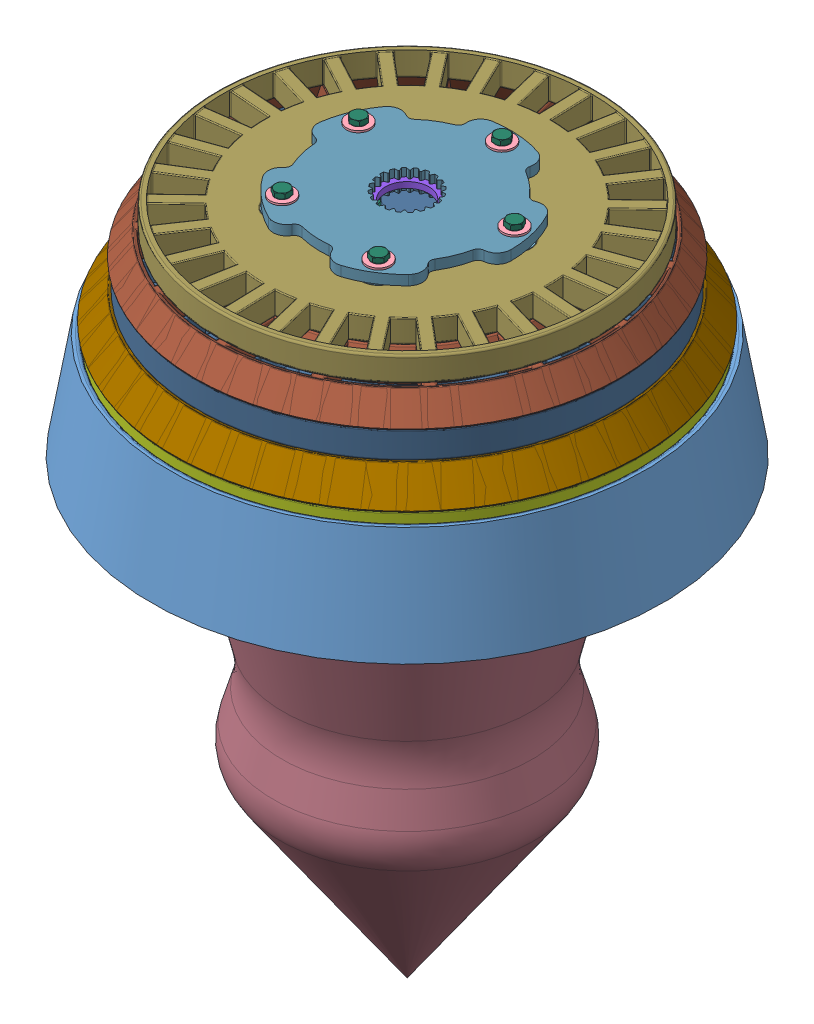
SolidWorks assembly Turbine Assembly, configuration Default. Lengths in mm.
Overall size (334.1 349.82 334.1).
50 component instances, 16 part files, 33 mates.
Components (placement in the parent):
- Turbine Fan 1-1: Turbine Fan 1 [Default] at (22.7534 150.4171 228.3834) size (259 53.75 259)
- needle roller bearing_nrba_iso-2: needle roller bearing_nrba_iso [ISO 1206-A - 493555 - 26,SI,NC,26] at (22.7534 136.5971 228.3834) x (0 -1 0) z (-0.182779 0 0.983154) size (20 55 55)
- Rear Turbine Hub-2: Rear Turbine Hub [Default] at (22.7534 170.4171 228.3834) x (-0.970998 0 0.239087) z (0 1 0) size (101.62 104.75 40.92)
- Turbine Link Assembly-1: Turbine Link Assembly [Default] at (-63.4742 236.9911 264.9834) x (0.691338 0 0.722532) z (0.722532 0 -0.691338) size (16 64.44 16)
  - Turbine Link-1: Turbine Link [Default] at (-7.9109 -2.865 69.2328) size (12 64.44 12)
  - Turbine Spacer 2-1: Turbine Spacer 2 [Default] at (-7.9109 3.135 69.2328) size (16 21.23 16)
  - Turbine Spacer-1: Turbine Spacer [Default] at (-7.9109 30.963 69.2328) size (16 23.35 16)
- Turbine Link Assembly-2: Turbine Link Assembly [Default] at (-38.7011 236.9911 157.6861) x (-0.473533 0 0.880776) z (0.880776 0 0.473533) size (16 64.44 16)
  - Turbine Link-1: Turbine Link [Default] at (-7.9109 -2.865 69.2328) size (12 64.44 12)
  - Turbine Spacer 2-1: Turbine Spacer 2 [Default] at (-7.9109 3.135 69.2328) size (16 21.23 16)
  - Turbine Spacer-1: Turbine Spacer [Default] at (-7.9109 30.963 69.2328) size (16 23.35 16)
- Turbine Link Assembly-3: Turbine Link Assembly [Default] at (71 236.9911 148.09) x (-0.983998 0 -0.178182) z (-0.178182 0 0.983998) size (16 64.44 16)
  - Turbine Link-1: Turbine Link [Default] at (-7.9109 -2.865 69.2328) size (12 64.44 12)
  - Turbine Spacer 2-1: Turbine Spacer 2 [Default] at (-7.9109 3.135 69.2328) size (16 21.23 16)
  - Turbine Spacer-1: Turbine Spacer [Default] at (-7.9109 30.963 69.2328) size (16 23.35 16)
- Turbine Link Assembly-4: Turbine Link Assembly [Default] at (114.026 236.9911 249.4566) x (-0.134611 0 -0.990899) z (-0.990899 0 0.134611) size (16 64.44 16)
  - Turbine Link-1: Turbine Link [Default] at (-7.9109 -2.865 69.2328) size (12 64.44 12)
  - Turbine Spacer 2-1: Turbine Spacer 2 [Default] at (-7.9109 3.135 69.2328) size (16 21.23 16)
  - Turbine Spacer-1: Turbine Spacer [Default] at (-7.9109 30.963 69.2328) size (16 23.35 16)
- Turbine Link Assembly-5: Turbine Link Assembly [Default] at (30.9163 236.9911 321.7007) x (0.900804 0 -0.434227) z (-0.434227 0 -0.900804) size (16 64.44 16)
  - Turbine Link-1: Turbine Link [Default] at (-7.9109 -2.865 69.2328) size (12 64.44 12)
  - Turbine Spacer 2-1: Turbine Spacer 2 [Default] at (-7.9109 3.135 69.2328) size (16 21.23 16)
  - Turbine Spacer-1: Turbine Spacer [Default] at (-7.9109 30.963 69.2328) size (16 23.35 16)
- Turbine Fan 2-1: Turbine Fan 2 [Default] at (22.7534 165.4171 228.3834) x (-0.07267 0 0.997356) z (-0.997356 0 -0.07267) size (234 15.68 234)
- Turbine Axis Spacer-1: Turbine Axis Spacer [Default] at (22.7534 234.8561 228.3834) x (0.984962 0 0.172768) z (0 -1 0) size (34 34 3)
- Turbine Fan 5.-1: Turbine Fan 5. [Default] at (22.7534 200.4171 228.3834) x (0 1 0) z (0.739195 0 -0.673491) size (15.2 236.5 236.5)
- Turbine Fan 3-2: Turbine Fan 3 [Default] at (22.7534 195.4171 228.3834) x (0.926086 0 0.377313) z (-0.377313 0 0.926086) size (212.5 14.22 212.5)
- Turbine Fan 6-1: Turbine Fan 6 [Default] at (22.7534 226.9171 228.3834) x (0 1 0) z (0.881108 0 0.472915) size (13.18 215 215)
- Turbine Fan 4-1: Turbine Fan 4 [Default] at (22.7534 233.9171 228.3834) x (0.926086 0 0.377313) z (0.377313 0 -0.926086) size (193 12.68 193)
- Turbine Housing-1: Turbine Housing [Default] at (22.7534 -107.1644 228.3834) x (0 1 0) z (0 0 -1) size (257.58 181.79 181.21)
- Front Turbine Hub-2: Front Turbine Hub [Default] at (22.7534 160.4171 228.3834) x (-0.07267 0 0.997356) z (0 1 0) size (101.62 104.75 10)
- hex screw gradeab_iso-2: hex screw gradeab_iso [ISO 4017 - M4 x 8-N] at (66.4483 157.6171 217.6245) x (0 1 0) z (-0.789962 0 -0.613155) size (10.8 8.08 7)
- hex screw gradeab_iso-3: hex screw gradeab_iso [ISO 4017 - M4 x 8-N] at (46.4882 157.6171 266.615) x (0 1 0) z (0.339034 0 -0.940774) size (10.8 8.08 7)
- hex screw gradeab_iso-4: hex screw gradeab_iso [ISO 4017 - M4 x 8-N] at (-6.2726 157.6171 262.7707) x (0 1 0) z (0.999497 0 0.031725) size (10.8 8.08 7)
- hex screw gradeab_iso-5: hex screw gradeab_iso [ISO 4017 - M4 x 8-N] at (-18.9204 157.6171 211.4043) x (0 1 0) z (0.278689 0 0.960381) size (10.8 8.08 7)
- hex screw gradeab_iso-6: hex screw gradeab_iso [ISO 4017 - M4 x 8-N] at (26.0236 157.6171 183.5023) x (0 1 0) z (-0.827257 0 0.561823) size (10.8 8.08 7)
- Front Turbine Hub-3: Front Turbine Hub [Default] at (22.7534 238.9171 228.3834) x (-0.970998 0 0.239087) z (0 -1 0) size (101.62 104.75 10)
- slotted capstan screw_din-2: slotted capstan screw_din [DIN 404 M6 x 8 --- 8N] at (-55.2466 131.9671 228.3834) x (0 1 0) z (0 0 -1) size (16.43 10 10)
- slotted capstan screw_din-4: slotted capstan screw_din [DIN 404 M6 x 8 --- 8N] at (-32.4009 131.9671 283.5377) x (0 1 0) z (-0.707107 0 -0.707107) size (16.43 10 10)
- slotted capstan screw_din-5: slotted capstan screw_din [DIN 404 M6 x 8 --- 8N] at (22.7534 131.9671 306.3834) x (0 1 0) z (-1 0 0) size (16.43 10 10)
- slotted capstan screw_din-6: slotted capstan screw_din [DIN 404 M6 x 8 --- 8N] at (77.9078 131.9671 283.5377) x (0 1 0) z (-0.707107 0 0.707107) size (16.43 10 10)
- slotted capstan screw_din-7: slotted capstan screw_din [DIN 404 M6 x 8 --- 8N] at (100.7534 131.9671 228.3834) x (0 1 0) z (0 0 1) size (16.43 10 10)
- slotted capstan screw_din-8: slotted capstan screw_din [DIN 404 M6 x 8 --- 8N] at (77.9078 131.9671 173.229) x (0 1 0) z (0.707107 0 0.707107) size (16.43 10 10)
- slotted capstan screw_din-9: slotted capstan screw_din [DIN 404 M6 x 8 --- 8N] at (22.7534 131.9671 150.3834) x (0 1 0) z (1 0 0) size (16.43 10 10)
- slotted capstan screw_din-10: slotted capstan screw_din [DIN 404 M6 x 8 --- 8N] at (-32.4009 131.9671 173.229) x (0 1 0) z (0.707107 0 -0.707107) size (16.43 10 10)
- hex screw gradeab_iso-7: hex screw gradeab_iso [ISO 4017 - M4 x 8-N] at (26.0236 242.6561 183.5023) x (0 -1 0) z (0.122239 0 0.992501) size (10.8 8.08 7)
- hex screw gradeab_iso-8: hex screw gradeab_iso [ISO 4017 - M4 x 8-N] at (-18.9204 242.6561 211.4043) x (0 -1 0) z (0.981698 0 0.190443) size (10.8 8.08 7)
- hex screw gradeab_iso-9: hex screw gradeab_iso [ISO 4017 - M4 x 8-N] at (-6.2726 242.6561 262.7707) x (0 -1 0) z (0.484484 0 -0.8748) size (10.8 8.08 7)
- hex screw gradeab_iso-10: hex screw gradeab_iso [ISO 4017 - M4 x 8-N] at (46.4882 242.6561 266.615) x (0 -1 0) z (-0.682271 0 -0.731099) size (10.8 8.08 7)
- hex screw gradeab_iso-11: hex screw gradeab_iso [ISO 4017 - M4 x 8-N] at (66.4483 242.6561 217.6245) x (0 -1 0) z (-0.90615 0 0.422956) size (10.8 8.08 7)
Mates (geometry in assembly coordinates):
- Coincident1: coincident anti-aligned: plane of Turbine Fan 1-1 through (22.7534 146.5971 228.3834) normal (0 -1 0); plane of needle roller bearing_nrba_iso-2 through (46.4597 146.5971 232.7906) normal (0 1 0)
- Concentric2: concentric aligned: cylinder of Turbine Fan 1-1 through (22.7534 146.5971 228.3834) axis (0 -1 0) radius 28; cylinder of needle roller bearing_nrba_iso-2 through (22.7534 144.5346 228.3834) axis (0 -1 0) radius 27.5
- Concentric4: concentric anti-aligned: cylinder of Turbine Fan 1-1 through (22.7534 175.9171 228.3834) axis (0 -1 0) radius 13; cylinder of Rear Turbine Hub-2 through (22.7534 142.6071 228.3834) axis (0 1 0) radius 11.5
- Concentric5: concentric anti-aligned: cylinder of needle roller bearing_nrba_iso-2 through (22.7534 144.5346 228.3834) axis (0 -1 0) radius 17.5; cylinder of Rear Turbine Hub-2 through (22.7534 142.6071 228.3834) axis (0 1 0) radius 9
- Concentric7: concentric anti-aligned: cylinder of Rear Turbine Hub-2 through (-18.9204 183.5251 211.4043) axis (0 -1 0) radius 2.5; cylinder of Turbine Link Assembly-1/Turbine Link-1 through (-18.9204 175.4171 211.4043) axis (0 1 0) radius 2.5
- Coincident8: coincident anti-aligned: plane of Rear Turbine Hub-2 through (22.7534 175.4171 228.3834) normal (0 1 0); plane of Turbine Link Assembly-1/Turbine Link-1 through (-18.9204 175.4171 211.4043) normal (0 -1 0)
- Concentric9: concentric aligned: cylinder of Rear Turbine Hub-2 through (22.7534 180.4171 228.3834) axis (0 -1 0) radius 32.5; cylinder of Turbine Fan 2-1 through (22.7534 180.4171 228.3834) axis (0 -1 0) radius 32.5
- Concentric10: concentric aligned: cylinder of Turbine Link Assembly-3/Turbine Spacer-1 through (66.4483 182.6771 217.6245) axis (0 1 0) radius 8; cylinder of Turbine Fan 2-1 through (66.4483 164.9171 217.6245) axis (0 1 0) radius 8
- Distance1: distance = 15 mm anti-aligned: plane of Rear Turbine Hub-2 through (22.7534 170.4171 228.3834) normal (0 -1 0); plane of Turbine Fan 1-1 through (22.7534 155.4171 228.3834) normal (0 1 0)
- Concentric13: concentric aligned: cone of Turbine Fan 1-1 through (22.7534 122.1645 228.3834) axis (0 1 0); cone of Turbine Fan 5.-1 through (22.7534 181.4171 228.3834) axis (0 1 0)
- Coincident15: coincident anti-aligned: plane of Turbine Fan 2-1 through (22.7534 180.4171 228.3834) normal (0 1 0); plane of Turbine Fan 5.-1 through (-29.6105 180.4171 170.9109) normal (0 -1 0)
- Concentric17: concentric aligned: cylinder of Turbine Fan 2-1 through (22.7534 180.4171 228.3834) axis (0 -1 0) radius 32.5; cylinder of Turbine Fan 3-2 through (22.7534 208.9171 228.3834) axis (0 -1 0) radius 32.5
- Concentric18: concentric aligned: cylinder of Turbine Link Assembly-2/Turbine Spacer-1 through (26.0236 182.6771 183.5023) axis (0 1 0) radius 8; cylinder of Turbine Fan 3-2 through (26.0236 194.8171 183.5023) axis (0 1 0) radius 8
- Coincident17: coincident anti-aligned: plane of Turbine Fan 3-2 through (22.7534 208.9171 228.3834) normal (0 1 0); plane of Turbine Fan 6-1 through (56.0939 208.9171 166.2652) normal (0 -1 0)
- Concentric20: concentric anti-aligned: cylinder of Turbine Fan 3-2 through (22.7534 208.9171 228.3834) axis (0 -1 0) radius 32.5; cylinder of Turbine Fan 4-1 through (22.7534 221.9171 228.3834) axis (0 1 0) radius 32.5
- Coincident18: coincident anti-aligned: plane of Turbine Fan 6-1 through (22.7534 221.9171 228.3834) normal (0 1 0); plane of Turbine Fan 4-1 through (22.7534 221.9171 228.3834) normal (0 -1 0)
- Coincident19: coincident anti-aligned: plane of Turbine Fan 1-1 through (22.7534 150.4171 228.3834) normal (0 -1 0); plane of Turbine Housing-1 through (77.9078 150.4171 283.5377) normal (0 1 0)
- Concentric22: concentric anti-aligned: cylinder of Turbine Fan 1-1 through (100.7534 175.9171 228.3834) axis (0 -1 0) radius 2.6; cylinder of Turbine Housing-1 through (100.7534 150.4171 228.3834) axis (0 1 0) radius 2.6
- Concentric23: concentric anti-aligned: cylinder of Turbine Fan 1-1 through (77.9078 175.9171 173.229) axis (0 -1 0) radius 2.6; cylinder of Turbine Housing-1 through (77.9078 150.4171 173.229) axis (0 1 0) radius 2.6
- Coincident21: coincident anti-aligned: plane of Turbine Fan 1-1 through (22.7534 165.4171 228.3834) normal (0 1 0); plane of Turbine Fan 2-1 through (22.7534 165.4171 228.3834) normal (0 -1 0)
- Coincident22: coincident anti-aligned: plane of Turbine Fan 5.-1 through (22.7534 195.4171 228.3834) normal (0 1 0); plane of Turbine Fan 3-2 through (22.7534 195.4171 228.3834) normal (0 -1 0)
- Concentric27: concentric anti-aligned: cylinder of Rear Turbine Hub-2 through (22.7534 142.6071 228.3834) axis (0 1 0) radius 9; cylinder of Front Turbine Hub-2 through (22.7534 165.4171 228.3834) axis (0 -1 0) radius 44
- Coincident25: coincident anti-aligned: plane of Turbine Fan 2-1 through (22.7534 165.4171 228.3834) normal (0 -1 0); plane of Front Turbine Hub-2 through (22.7534 165.4171 228.3834) normal (0 1 0)
- Concentric28: concentric aligned: cylinder of Rear Turbine Hub-2 through (66.4483 183.5251 217.6245) axis (0 -1 0) radius 2.5; cylinder of Front Turbine Hub-2 through (66.4483 170.4171 217.6245) axis (0 -1 0) radius 2.5
- Concentric29: concentric aligned: cylinder of Rear Turbine Hub-2 through (66.4483 183.5251 217.6245) axis (0 -1 0) radius 2.5; cylinder of hex screw gradeab_iso-2 through (66.4483 157.6171 217.6245) axis (0 -1 0) radius 2
- Coincident26: coincident anti-aligned: plane of Front Turbine Hub-2 through (22.7534 160.4171 228.3834) normal (0 -1 0); plane of hex screw gradeab_iso-2 through (68.9264 160.4171 214.4319) normal (0 1 0)
- Concentric30: concentric aligned: cylinder of Turbine Fan 4-1 through (22.7534 221.9171 228.3834) axis (0 1 0) radius 32.5; cylinder of Front Turbine Hub-3 through (22.7534 228.9171 228.3834) axis (0 1 0) radius 32.5
- Coincident27: coincident anti-aligned: plane of Turbine Fan 4-1 through (22.7534 233.9171 228.3834) normal (0 1 0); plane of Front Turbine Hub-3 through (22.7534 233.9171 228.3834) normal (0 -1 0)
- Concentric31: concentric aligned: cylinder of Turbine Link Assembly-1/Turbine Link-1 through (-18.9204 175.4171 211.4043) axis (0 1 0) radius 2.5; cylinder of Front Turbine Hub-3 through (-18.9204 228.9171 211.4043) axis (0 1 0) radius 2.5
- Coincident28: coincident anti-aligned: plane of Turbine Housing-1 through (-55.2466 140.4171 228.3834) normal (0 -1 0); plane of slotted capstan screw_din-2 through (-50.2466 140.4171 228.3834) normal (0 1 0)
- Concentric35: concentric anti-aligned: cylinder of Turbine Housing-1 through (-55.2466 150.4171 228.3834) axis (0 1 0) radius 2.6; cylinder of slotted capstan screw_din-2 through (-55.2466 100.2171 228.3834) axis (0 -1 0) radius 3
- Concentric36: concentric aligned: cylinder of Turbine Link Assembly-2/Turbine Link-1 through (26.0236 175.4171 183.5023) axis (0 1 0) radius 2.5; cylinder of hex screw gradeab_iso-7 through (26.0236 242.6561 183.5023) axis (0 1 0) radius 2
- Coincident29: coincident anti-aligned: plane of Turbine Link Assembly-2/Turbine Link-1 through (26.0236 239.8561 183.5023) normal (0 1 0); plane of hex screw gradeab_iso-7 through (30.0347 239.8561 183.0083) normal (0 -1 0)
